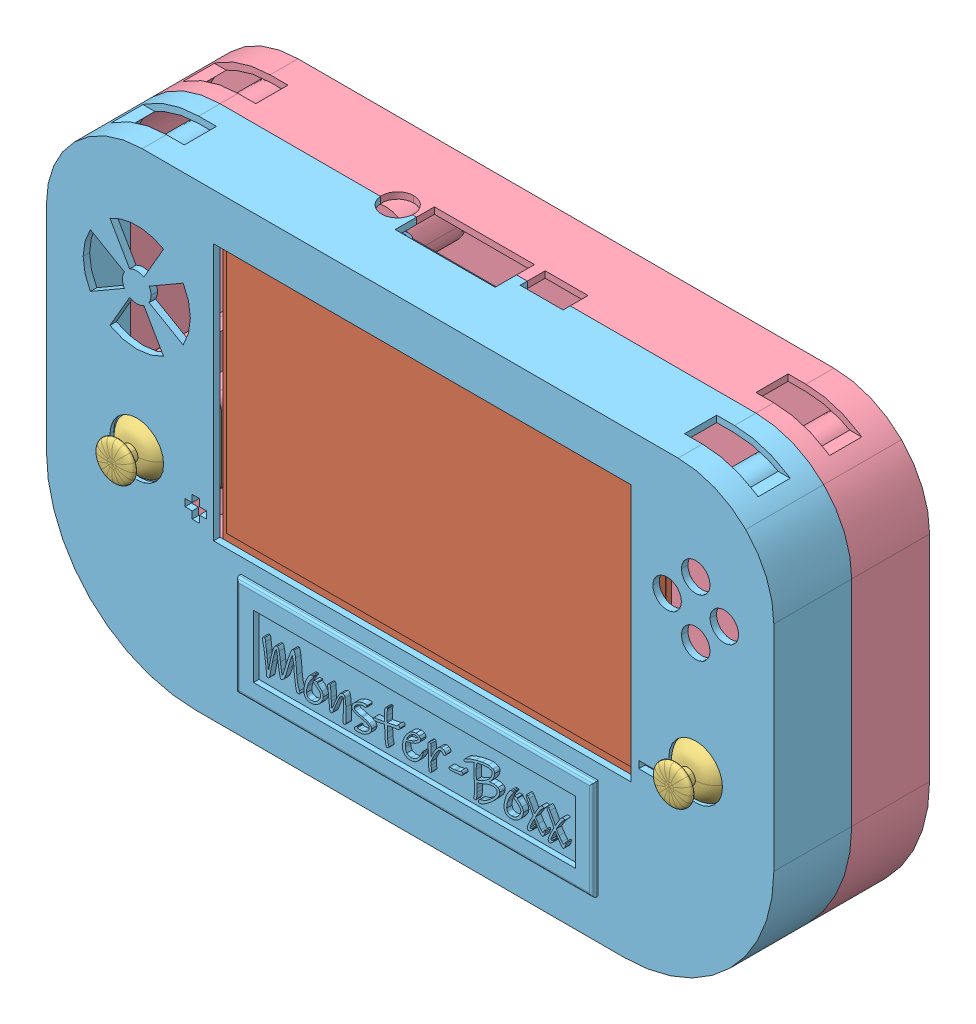
SolidWorks assembly LOKUM, configuration Default. Lengths in mm.
Overall size (203.6 128.6 51.05).
10 component instances, 5 part files, 0 mates.
Components (placement in the parent):
- LOKUM.STEP-1: LOKUM.STEP [Default] at origin size (203.6 128.6 51.05)
  - LOKUM.STEP.STEP-1: LOKUM.STEP.STEP [Default] at origin size (203.6 128.6 51.05)
    - Monster-Boxx v8.step.STEP.STEP-1: Monster-Boxx v8.step.STEP.STEP [Default] at origin size (203.6 128.6 51.05)
      - RPi3B+ and 5inch LCD.step.STEP.STEP-1: RPi3B+ and 5inch LCD.step.STEP.STEP [Default] at (40 80 80) x (-1 0 0) z (0 1 0) size (123.14 23.17 80.4)
        - Rpi3Bplus.step.STEP.STEP-1: Rpi3Bplus.step.STEP.STEP [Default] at (-87.8742 -65 36.0456) size (87.03 17.52 58.47)
        - Waveshare_5inch_HDMI_LCD_V2_v12.step.STEP.STEP-1: Waveshare_5inch_HDMI_LCD_V2_v12.step.STEP.STEP [Default] at (-63.4292 -47.4434 -2.9194) x (-1 0 0) z (0 1 0) size (121.11 77.93 5.59)
      - JoyStick v10.step.STEP.STEP-1: JoyStick v10.step.STEP.STEP [Default] at (23.517 53.275 29.5747) size (22.85 22.8 19.25)
      - JoyStick v10.step.STEP.STEP-2: JoyStick v10.step.STEP.STEP [Default] at (179.9704 53.3041 30) size (22.85 22.8 19.25)
      - Monster-Boxx.step.STEP.STEP-1: Monster-Boxx.step.STEP.STEP [Default] at origin size (203.6 128.6 31.8)
      - Monster-Boxx-0.step.STEP.STEP-1: Monster-Boxx-0.step.STEP.STEP [Default] at origin size (203.6 128.6 23.3)
